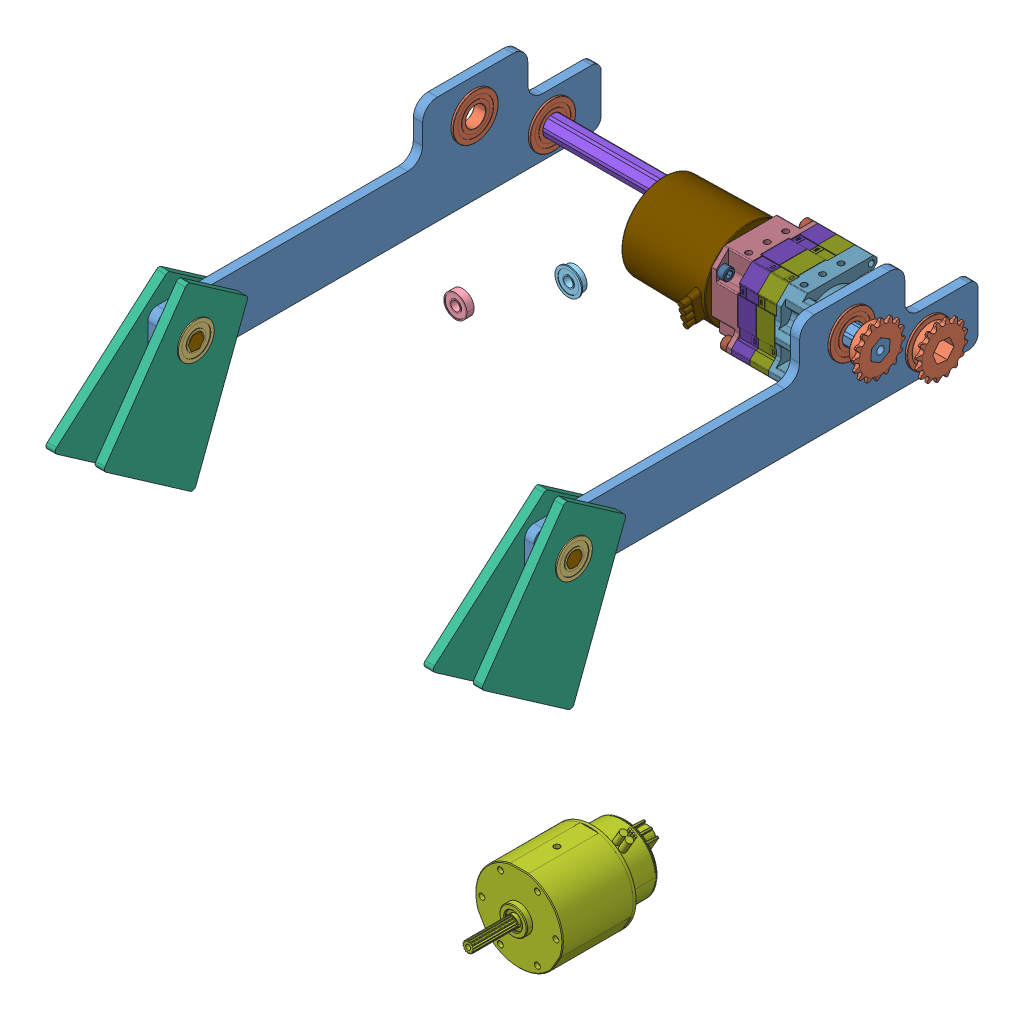
SolidWorks assembly yesthisone, configuration Default. Lengths in mm.
Overall size (933.45 166.15 369.14).
60 component instances, 20 part files, 42 mates.
Components (placement in the parent):
- arm_attached_to_base-1: arm_attached_to_base [Default] at (59.2501 122.8758 287.3153) size (6.35 73.97 304.8)
- 217-4006_0_500_flanged_thunderhex_bearing.step-1: 217-4006_0_500_flanged_thunderhex_bearing.step [Default] at (63.2189 91.0834 17.049) x (0 0 -1) z (1 0 0) size (31.12 31.12 7.94)
- 217-5829_0375_flanged_thunderhex_bearing.step-1: 217-5829_0375_flanged_thunderhex_bearing.step [Default] at (58.4881 91.0834 267.4195) size (7.11 24.61 24.61)
- WCP-0041_0_250_radial_bearing.step-1: WCP-0041_0_250_radial_bearing.step [Default] at (73.6016 23.6501 88.0497) size (15.88 15.88 4.98) (hidden)
- WCP-0042_0_250_flanged_bearing.step-1: WCP-0042_0_250_flanged_bearing.step [Default] at (78.0739 3.6818 15.0138) size (18.24 18.24 4.98) (hidden)
- 217-4006_0_500_flanged_thunderhex_bearing.step-2: 217-4006_0_500_flanged_thunderhex_bearing.step [Default] at (63.2189 122.8758 70.1046) x (0 0 -1) z (1 0 0) size (31.12 31.12 7.94)
- geezman-1: geezman [Default] at (131.9281 12.0134 290.3608) x (0 0.571393 0.820677) z (-1 0 0) size (76.26 101.6 7.11)
  - base_piece_ohne_bearing-1: base_piece_ohne_bearing [Default] at (0.9527 105.2192 73.4399) size (76.26 101.6 6.35)
  - WCP-0042_0_250_flanged_bearing.step-1: WCP-0042_0_250_flanged_bearing.step [Default] at (26.3527 77.9995 75.9291) size (18.24 18.24 4.98) (hidden)
  - 217-4006_0_500_flanged_thunderhex_bearing.step-1: 217-4006_0_500_flanged_thunderhex_bearing.step [Default] at (107.3505 72.9189 87.3707) size (31.12 31.12 7.94) (hidden)
  - 217-5829_0375_flanged_thunderhex_bearing.step-1: 217-5829_0375_flanged_thunderhex_bearing.step [Default] at (26.3527 77.9995 80.5519) x (0 0 -1) z (1 0 0) size (7.11 24.61 24.61)
  - WCP-0041_0_250_radial_bearing.step-1: WCP-0041_0_250_radial_bearing.step [Default] at (93.1971 45.2789 84.007) size (15.88 15.88 4.98) (hidden)
  - WCP-0042_0_250_flanged_bearing.step-2: WCP-0042_0_250_flanged_bearing.step [Default] at (68.101 81.3251 81.4434) size (18.24 18.24 4.98) (hidden)
- geezman-2: geezman [Default] at (251.6847 42.1288 333.6148) x (0 -0.571393 -0.820677) z (1 0 0) size (76.26 101.6 7.11)
  - base_piece_ohne_bearing-1: base_piece_ohne_bearing [Default] at (0.9527 105.2192 73.4399) size (76.26 101.6 6.35)
  - WCP-0042_0_250_flanged_bearing.step-1: WCP-0042_0_250_flanged_bearing.step [Default] at (26.3527 77.9995 75.9291) size (18.24 18.24 4.98) (hidden)
  - 217-4006_0_500_flanged_thunderhex_bearing.step-1: 217-4006_0_500_flanged_thunderhex_bearing.step [Default] at (107.3505 72.9189 87.3707) size (31.12 31.12 7.94) (hidden)
  - 217-5829_0375_flanged_thunderhex_bearing.step-1: 217-5829_0375_flanged_thunderhex_bearing.step [Default] at (26.3527 77.9995 80.5519) x (0 0 -1) z (1 0 0) size (7.11 24.61 24.61)
  - WCP-0041_0_250_radial_bearing.step-1: WCP-0041_0_250_radial_bearing.step [Default] at (93.1971 45.2789 84.007) size (15.88 15.88 4.98) (hidden)
  - WCP-0042_0_250_flanged_bearing.step-2: WCP-0042_0_250_flanged_bearing.step [Default] at (68.101 81.3251 81.4434) size (18.24 18.24 4.98) (hidden)
- arm_attached_to_base-2: arm_attached_to_base [Default] at (318.0126 122.8758 287.3153) size (6.35 73.97 304.8)
- 217-4006_0_500_flanged_thunderhex_bearing.step-3: 217-4006_0_500_flanged_thunderhex_bearing.step [Default] at (321.9814 122.8758 70.1046) x (0 0 -1) z (1 0 0) size (31.12 31.12 7.94)
- 217-4006_0_500_flanged_thunderhex_bearing.step-4: 217-4006_0_500_flanged_thunderhex_bearing.step [Default] at (321.9814 91.0834 17.049) x (0 0 -1) z (1 0 0) size (31.12 31.12 7.94)
- 217-5829_0375_flanged_thunderhex_bearing.step-2: 217-5829_0375_flanged_thunderhex_bearing.step [Default] at (325.1246 91.0834 267.4195) x (-1 0 0) z (0 -0.924225 -0.381849) size (7.11 24.61 24.61)
- 217-6515_Falcon_500_Default_As Machined_.step-1: 217-6515_Falcon_500_Default_As Machined_.step [Default] at (441.1952 5.6754 388.3022) size (60 60 115.81) (hidden)
- correct stock-2: correct stock [Default] at (-131.2499 91.0834 17.049) x (0 -0.924225 -0.381849) z (1 0 0) size (19.87 18.09 914.4)
- geezman-3: geezman [Default] at (-7.8398 42.1288 333.6148) x (0 -0.571393 -0.820677) z (1 0 0) size (76.26 101.6 7.11)
  - base_piece_ohne_bearing-1: base_piece_ohne_bearing [Default] at (0.9527 105.2192 73.4399) size (76.26 101.6 6.35)
  - WCP-0042_0_250_flanged_bearing.step-1: WCP-0042_0_250_flanged_bearing.step [Default] at (26.3527 77.9995 75.9291) size (18.24 18.24 4.98) (hidden)
  - 217-4006_0_500_flanged_thunderhex_bearing.step-1: 217-4006_0_500_flanged_thunderhex_bearing.step [Default] at (107.3505 72.9189 87.3707) size (31.12 31.12 7.94) (hidden)
  - 217-5829_0375_flanged_thunderhex_bearing.step-1: 217-5829_0375_flanged_thunderhex_bearing.step [Default] at (26.3527 77.9995 80.5519) x (0 0 -1) z (1 0 0) size (7.11 24.61 24.61)
  - WCP-0041_0_250_radial_bearing.step-1: WCP-0041_0_250_radial_bearing.step [Default] at (93.1971 45.2789 84.007) size (15.88 15.88 4.98) (hidden)
  - WCP-0042_0_250_flanged_bearing.step-2: WCP-0042_0_250_flanged_bearing.step [Default] at (68.101 81.3251 81.4434) size (18.24 18.24 4.98) (hidden)
- geezman-4: geezman [Default] at (391.4526 12.0134 290.3608) x (0 0.571393 0.820677) z (-1 0 0) size (76.26 101.6 7.11)
  - base_piece_ohne_bearing-1: base_piece_ohne_bearing [Default] at (0.9527 105.2192 73.4399) size (76.26 101.6 6.35)
  - WCP-0042_0_250_flanged_bearing.step-1: WCP-0042_0_250_flanged_bearing.step [Default] at (26.3527 77.9995 75.9291) size (18.24 18.24 4.98) (hidden)
  - 217-4006_0_500_flanged_thunderhex_bearing.step-1: 217-4006_0_500_flanged_thunderhex_bearing.step [Default] at (107.3505 72.9189 87.3707) size (31.12 31.12 7.94) (hidden)
  - 217-5829_0375_flanged_thunderhex_bearing.step-1: 217-5829_0375_flanged_thunderhex_bearing.step [Default] at (26.3527 77.9995 80.5519) x (0 0 -1) z (1 0 0) size (7.11 24.61 24.61)
  - WCP-0041_0_250_radial_bearing.step-1: WCP-0041_0_250_radial_bearing.step [Default] at (93.1971 45.2789 84.007) size (15.88 15.88 4.98) (hidden)
  - WCP-0042_0_250_flanged_bearing.step-2: WCP-0042_0_250_flanged_bearing.step [Default] at (68.101 81.3251 81.4434) size (18.24 18.24 4.98) (hidden)
- hex_shaft-1: hex_shaft [Default] at (491.8121 90.3396 267.5181) x (0 -0.924225 -0.381849) z (1 0 0) size (10.81 9.5 38.1)
- hex_shaft-2: hex_shaft [Default] at (751.3366 91.0075 267.49) x (0 -0.924225 -0.381849) z (1 0 0) size (10.81 9.5 38.1)
- MAXPlanetary 2-Stage-1: MAXPlanetary 2-Stage [Default] at (264.0376 122.8978 70.1041) x (0 0 -1) z (1 0 0) size (89.61 89.51 122.08)
  - MAXPlanetary 2-Stage.STEP-1: MAXPlanetary 2-Stage.STEP [Default] at origin size (89.61 89.51 122.08)
    - REV-25-2109_2-Stage (No Shaft, For NEO).STEP-1: REV-25-2109_2-Stage (No Shaft, For NEO).STEP [Default] at origin size (65.15 54.03 73.34)
      - REV-25-2107_2-Stage.STEP-1: REV-25-2107_2-Stage.STEP [Default] at (0 0 6.35) x (-1 0 0) z (0 0 -1) size (65.15 54.03 73.34)
        - #10 Socket Head Cap Screws_0.500in Long.STEP-1: #10 Socket Head Cap Screws_0.500in Long.STEP [Default] at (21.1355 14.0872 12.7) x (0.923728 0.383049 0) z (0.383049 -0.923728 0) size (7.94 17.53 7.94)
        - #10 Socket Head Cap Screws_0.500in Long.STEP-2: #10 Socket Head Cap Screws_0.500in Long.STEP [Default] at (-21.1355 -14.0872 12.7) x (0.923728 0.383049 0) z (0.383049 -0.923728 0) size (7.94 17.53 7.94)
        - #10 Socket Head Cap Screws_1.500in Long.STEP-1: #10 Socket Head Cap Screws_1.500in Long.STEP [Default] at (-26.9919 21.4312 0) x (0.777574 0.628792 0) z (-0.628792 0.777574 0) size (7.94 42.93 7.94)
        - #10 Socket Head Cap Screws_1.500in Long.STEP-2: #10 Socket Head Cap Screws_1.500in Long.STEP [Default] at (26.9919 -21.4312 0) x (0.777574 0.628792 0) z (-0.628792 0.777574 0) size (7.94 42.93 7.94)
        - #10-32 Button Head Cap Screws_0.500in Long.STEP-1: #10-32 Button Head Cap Screws_0.500in Long.STEP [Default] at (0 0 -35.2425) x (0.655967 -0.754789 0) z (-0.754789 -0.655967 0) size (9.17 15.27 9.17)
      - REV-21-2106.STEP-1: REV-21-2106.STEP [Default] at origin size (61.91 50.8 19.05)
      - REV-21-2104.STEP-1: REV-21-2104.STEP [Default] at (0 0 44.45) x (0 0 1) z (-1 0 0) size (23.2 50.8 61.92)
      - REV-21-2108.STEP-1: REV-21-2108.STEP [Default] at (0 0 7.0985) x (-0.554615 -0.832107 0) z (0 0 -1) size (25.4 25.4 14.94)
    - REV-21-2101.STEP-1: REV-21-2101.STEP [Default] at (0 0 28.575) size (61.91 50.8 16.85)
    - REV-21-2102.STEP-1: REV-21-2102.STEP [Default] at (0 0 15.875) size (61.91 50.8 16.85)
    - REV-21-1650.STEP-1: REV-21-1650.STEP [Default] at (0 0 -9.525) x (0.554615 0.832107 0) z (0 0 1) size (64.41 64.76 93.26)
- correct stock - Copy-1: correct stock - Copy [Default] at (-112.1999 122.8758 70.1046) x (0 0.481071 -0.876682) z (1 0 0) size (19.87 18.09 914.4)
- 16T_#25_500_hex_hubbed_sprocket_217-2642-1: 16T_#25_500_hex_hubbed_sprocket_217-2642 [Default] at (332.3319 91.0718 17.0579) x (0 0.381849 -0.924225) z (1 0 0) size (35.21 35.21 9.18)
- 16T_#25_500_hex_hubbed_sprocket_217-2642-2: 16T_#25_500_hex_hubbed_sprocket_217-2642 [Default] at (342.2061 122.8682 70.0921) x (0 -0.876682 -0.481071) z (1 0 0) size (35.21 35.21 9.18)
Mates (geometry in assembly coordinates):
- Concentric1: concentric anti-aligned: cylinder of arm_attached_to_base-1 through (65.6001 91.0834 17.049) axis (-1 0 0) radius 14.224; cylinder of 217-4006_0_500_flanged_thunderhex_bearing.step-1 through (116.4678 91.0834 17.049) axis (1 0 0) radius 14.2875
- Coincident1: coincident aligned: plane of arm_attached_to_base-1 through (59.2501 122.8758 287.3153) normal (-1 0 0); plane of 217-4006_0_500_flanged_thunderhex_bearing.step-1 through (59.2501 103.3709 17.049) normal (-1 0 0)
- Concentric2: concentric anti-aligned: cylinder of arm_attached_to_base-1 through (65.6001 122.8758 70.1046) axis (-1 0 0) radius 14.224; cylinder of 217-4006_0_500_flanged_thunderhex_bearing.step-2 through (116.4678 122.8758 70.1046) axis (1 0 0) radius 14.2875
- Coincident2: coincident aligned: plane of arm_attached_to_base-1 through (59.2501 122.8758 287.3153) normal (-1 0 0); plane of 217-4006_0_500_flanged_thunderhex_bearing.step-2 through (59.2501 135.1633 70.1046) normal (-1 0 0)
- Concentric3: concentric aligned: cylinder of arm_attached_to_base-1 through (65.6001 91.0834 267.4195) axis (-1 0 0) radius 11.176; cylinder of 217-5829_0375_flanged_thunderhex_bearing.step-1 through (58.4881 91.0834 267.4195) axis (-1 0 0) radius 11.1125
- Coincident3: coincident aligned: plane of arm_attached_to_base-1 through (65.6001 122.8758 287.3153) normal (1 0 0); plane of 217-5829_0375_flanged_thunderhex_bearing.step-1 through (65.6001 100.9894 267.4195) normal (1 0 0)
- Coincident4: coincident anti-aligned: plane of 217-5829_0375_flanged_thunderhex_bearing.step-1 through (58.4881 97.7084 267.4195) normal (-1 0 0); plane of geezman-1/217-5829_0375_flanged_thunderhex_bearing.step-1 through (58.4881 95.2894 264.4911) normal (1 0 0)
- Concentric4: concentric aligned: cylinder of 217-5829_0375_flanged_thunderhex_bearing.step-1 through (58.4881 91.0834 267.4195) axis (-1 0 0) radius 5.125; cylinder of geezman-1/217-5829_0375_flanged_thunderhex_bearing.step-1 through (51.3761 91.0834 267.4195) axis (-1 0 0) radius 5.125
- Concentric5: concentric anti-aligned: cylinder of arm_attached_to_base-2 through (324.3626 122.8758 70.1046) axis (-1 0 0) radius 14.224; cylinder of 217-4006_0_500_flanged_thunderhex_bearing.step-3 through (375.2303 122.8758 70.1046) axis (1 0 0) radius 14.2875
- Coincident5: coincident aligned: plane of arm_attached_to_base-2 through (318.0126 122.8758 287.3153) normal (-1 0 0); plane of 217-4006_0_500_flanged_thunderhex_bearing.step-3 through (318.0126 135.1633 70.1046) normal (-1 0 0)
- Concentric6: concentric anti-aligned: cylinder of arm_attached_to_base-2 through (324.3626 91.0834 17.049) axis (-1 0 0) radius 14.224; cylinder of 217-4006_0_500_flanged_thunderhex_bearing.step-4 through (375.2303 91.0834 17.049) axis (1 0 0) radius 14.2875
- Coincident6: coincident aligned: plane of arm_attached_to_base-2 through (318.0126 122.8758 287.3153) normal (-1 0 0); plane of 217-4006_0_500_flanged_thunderhex_bearing.step-4 through (318.0126 103.3709 17.049) normal (-1 0 0)
- Coincident7: coincident aligned: plane of arm_attached_to_base-2 through (318.0126 122.8758 287.3153) normal (-1 0 0); plane of 217-5829_0375_flanged_thunderhex_bearing.step-2 through (318.0126 94.866 258.2641) normal (-1 0 0)
- Concentric7: concentric anti-aligned: cylinder of arm_attached_to_base-2 through (324.3626 91.0834 267.4195) axis (-1 0 0) radius 11.176; cylinder of 217-5829_0375_flanged_thunderhex_bearing.step-2 through (325.1246 91.0834 267.4195) axis (1 0 0) radius 11.1125
- Coincident8: coincident anti-aligned: plane of geezman-2/217-5829_0375_flanged_thunderhex_bearing.step-1 through (325.1246 95.2894 264.4911) normal (-1 0 0); plane of 217-5829_0375_flanged_thunderhex_bearing.step-2 through (325.1246 93.6132 261.2965) normal (1 0 0)
- Concentric8: concentric aligned: cylinder of geezman-2/217-5829_0375_flanged_thunderhex_bearing.step-1 through (332.2366 91.0834 267.4195) axis (1 0 0) radius 5.125; cylinder of 217-5829_0375_flanged_thunderhex_bearing.step-2 through (325.1246 91.0834 267.4195) axis (1 0 0) radius 5.125
- Coincident11: coincident aligned: plane of 217-4006_0_500_flanged_thunderhex_bearing.step-1 through (59.2501 97.9584 17.049) normal (-1 0 0); plane of correct stock-2 through (59.2501 91.0834 17.049) normal (-1 0 0)
- Concentric10: concentric aligned: cylinder of 217-4006_0_500_flanged_thunderhex_bearing.step-1 through (116.4678 91.0834 17.049) axis (1 0 0) radius 6.875; cylinder of correct stock-2 through (-588.4499 91.0834 17.049) axis (1 0 0) radius 6.87
- Concentric11: concentric aligned: cylinder of 217-4006_0_500_flanged_thunderhex_bearing.step-4 through (375.2303 91.0834 17.049) axis (1 0 0) radius 6.875; cylinder of correct stock-2 through (-588.4499 91.0834 17.049) axis (1 0 0) radius 6.87
- Coincident12: coincident aligned: plane of 217-4006_0_500_flanged_thunderhex_bearing.step-4 through (325.9501 100.6854 17.049) normal (1 0 0); plane of correct stock-2 through (325.9501 91.0834 17.049) normal (1 0 0)
- Coincident13: coincident anti-aligned: plane of 217-5829_0375_flanged_thunderhex_bearing.step-2 through (318.0126 93.0404 262.6828) normal (-1 0 0); plane of geezman-4/217-5829_0375_flanged_thunderhex_bearing.step-1 through (318.0126 95.2894 264.4911) normal (1 0 0)
- Concentric12: concentric anti-aligned: cylinder of 217-5829_0375_flanged_thunderhex_bearing.step-2 through (325.1246 91.0834 267.4195) axis (1 0 0) radius 5.125; cylinder of geezman-4/217-5829_0375_flanged_thunderhex_bearing.step-1 through (310.9006 91.0834 267.4195) axis (-1 0 0) radius 5.125
- Coincident14: coincident anti-aligned: plane of 217-5829_0375_flanged_thunderhex_bearing.step-1 through (65.6001 96.2084 267.4195) normal (1 0 0); plane of geezman-3/217-5829_0375_flanged_thunderhex_bearing.step-1 through (65.6001 95.2894 264.4911) normal (-1 0 0)
- Concentric13: concentric anti-aligned: cylinder of 217-5829_0375_flanged_thunderhex_bearing.step-1 through (58.4881 91.0834 267.4195) axis (-1 0 0) radius 5.125; cylinder of geezman-3/217-5829_0375_flanged_thunderhex_bearing.step-1 through (72.7121 91.0834 267.4195) axis (1 0 0) radius 5.125
- Coincident15: coincident aligned: plane of geezman-1/base_piece_ohne_bearing-1 through (52.1381 15.5279 289.0746) normal (0 -0.820677 0.571393); plane of geezman-3/base_piece_ohne_bearing-1 through (71.9501 44.5547 330.765) normal (0 -0.820677 0.571393)
- Coincident16: coincident aligned: plane of geezman-2/base_piece_ohne_bearing-1 through (331.4746 44.5547 330.765) normal (0 -0.820677 0.571393); plane of geezman-4/base_piece_ohne_bearing-1 through (311.6626 15.5279 289.0746) normal (0 -0.820677 0.571393)
- Coincident18: coincident aligned: plane of geezman-3/base_piece_ohne_bearing-1 through (71.9501 44.5547 330.765) normal (0 -0.820677 0.571393); plane of geezman-4/base_piece_ohne_bearing-1 through (311.6626 15.5279 289.0746) normal (0 -0.820677 0.571393)
- Coincident19: coincident aligned: plane of geezman-3/217-5829_0375_flanged_thunderhex_bearing.step-1 through (72.7121 96.5204 263.634) normal (1 0 0); plane of hex_shaft-1 through (72.7121 90.3396 267.5181) normal (1 0 0)
- Tangent6: tangent aligned: cylinder of 217-5829_0375_flanged_thunderhex_bearing.step-1 through (58.4881 91.0834 267.4195) axis (-1 0 0) radius 5.125; plane of hex_shaft-1 through (949.0121 91.0603 272.9551) normal (0 -0.381849 0.924225)
- Tangent7: tangent aligned: cylinder of geezman-3/217-5829_0375_flanged_thunderhex_bearing.step-1 through (72.7121 91.0834 267.4195) axis (1 0 0) radius 5.125; plane of hex_shaft-1 through (949.0121 85.2706 265.4238) normal (0 -0.609477 -0.792804)
- Coincident21: coincident aligned: plane of geezman-2/217-5829_0375_flanged_thunderhex_bearing.step-1 through (332.2366 96.5204 263.634) normal (1 0 0); plane of hex_shaft-2 through (332.2366 91.0075 267.49) normal (1 0 0)
- Coincident27: coincident anti-aligned: line of MAXPlanetary 2-Stage-1/MAXPlanetary 2-Stage.STEP-1/REV-25-2109_2-Stage (No Shaft, For NEO).STEP-1/REV-21-2104.STEP-1 through (306.9001 126.4287 63.6696) axis (0 0.518693 0.85496); line of correct stock - Copy-1 through (306.9001 129.6541 68.986) axis (0 -0.518693 -0.85496)
- Coincident28: coincident anti-aligned: plane of MAXPlanetary 2-Stage-1/MAXPlanetary 2-Stage.STEP-1/REV-25-2109_2-Stage (No Shaft, For NEO).STEP-1/REV-21-2104.STEP-1 through (306.9001 122.8978 70.1041) normal (1 0 0); plane of correct stock - Copy-1 through (306.9001 122.8758 70.1046) normal (-1 0 0)
- Coincident29: coincident anti-aligned: line of MAXPlanetary 2-Stage-1/MAXPlanetary 2-Stage.STEP-1/REV-25-2109_2-Stage (No Shaft, For NEO).STEP-1/REV-21-2104.STEP-1 through (306.9001 130.2358 69.9447) axis (0 -0.481071 0.876682); line of correct stock - Copy-1 through (306.9001 127.2337 75.4155) axis (0 0.481071 -0.876682)
- Coincident31: coincident anti-aligned: plane of arm_attached_to_base-2 through (318.0126 122.8758 287.3153) normal (-1 0 0); plane of MAXPlanetary 2-Stage-1/MAXPlanetary 2-Stage.STEP-1/REV-25-2109_2-Stage (No Shaft, For NEO).STEP-1/REV-21-2104.STEP-1 through (318.0126 122.8978 70.1041) normal (1 0 0)
- Concentric21: concentric aligned: cylinder of 217-4006_0_500_flanged_thunderhex_bearing.step-3 through (375.2303 122.8758 70.1046) axis (1 0 0) radius 6.875; cylinder of correct stock - Copy-1 through (-569.3999 122.8758 70.1046) axis (1 0 0) radius 6.87
- Coincident32: coincident aligned: plane of correct stock - Copy-1 through (345.0001 122.8758 70.1046) normal (1 0 0); plane of 16T_#25_500_hex_hubbed_sprocket_217-2642-2 through (345.0001 122.8682 70.0921) normal (1 0 0)
- Coincident33: coincident anti-aligned: plane of correct stock - Copy-1 through (345.0001 115.5159 70.2645) normal (0 -0.876682 -0.481071); plane of 16T_#25_500_hex_hubbed_sprocket_217-2642-2 through (335.8234 115.5229 70.2516) normal (0 0.876682 0.481071)
- Coincident34: coincident anti-aligned: plane of correct stock - Copy-1 through (345.0001 119.0574 63.8107) normal (0 -0.021721 -0.999764); plane of 16T_#25_500_hex_hubbed_sprocket_217-2642-2 through (335.8234 119.0574 63.8107) normal (0 0.021721 0.999764)
- Coincident35: coincident anti-aligned: plane of 217-4006_0_500_flanged_thunderhex_bearing.step-4 through (325.9501 100.6854 17.049) normal (1 0 0); plane of 16T_#25_500_hex_hubbed_sprocket_217-2642-1 through (325.9501 91.0718 17.0579) normal (-1 0 0)
- Coincident36: coincident anti-aligned: plane of correct stock-2 through (325.9501 92.0509 24.3468) normal (0 -0.381849 0.924225); plane of 16T_#25_500_hex_hubbed_sprocket_217-2642-1 through (325.9491 92.0374 24.3412) normal (0 0.381849 -0.924225)
- Coincident37: coincident anti-aligned: plane of correct stock-2 through (325.9501 85.2471 21.5357) normal (0 -0.991327 0.131421); plane of 16T_#25_500_hex_hubbed_sprocket_217-2642-1 through (325.9491 85.2471 21.5357) normal (0 0.991327 -0.131421)
